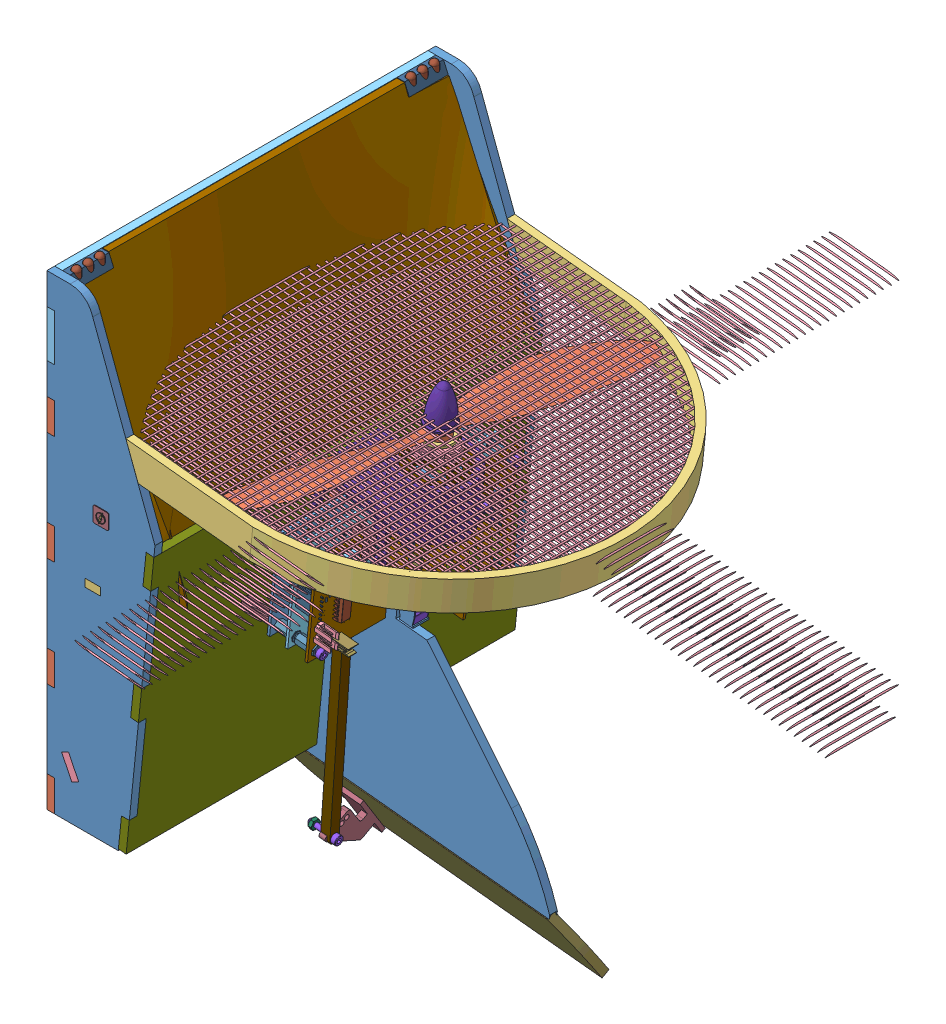
SolidWorks assembly AssTotaleSimu4, configuration Défaut. Lengths in mm. (continued)
Components (placement in the parent): (continued)
- AssStructSimu-1: AssStructSimu [Défaut] at (-125.7658 -1.8483 624.6548) x (1 0 0) z (0 0 -1) size (253.25 324.59 251.6) (continued)
  - AssCarte-1: AssCarte [Défaut] at (38.0121 147.1029 290.772) x (-0.101852 0.9948 0) z (0.9948 0.101852 0) size (66.52 130.57 98.72) (continued)
    - carte_onduleur_v3-1: carte_onduleur_v3 [Défaut] at (-131.8199 12.0892 20.7912) size (66.52 130.57 82.34) (continued)
      - U_DSPIC-1: U_DSPIC [Défaut] at (1.863 -2.61 0.803) size (7.92 35.56 7.75)
        - Open CASCADE STEP translator 6.8 1.17.1-1: Open CASCADE STEP translator 6.8 1.17.1 [Défaut] at origin size (7.92 35.56 7.75)
          - Body_1_4-1: Body_1_4 [Défaut] at (0 -0.2 4) x (1 0 0) z (0 -1 0) size (7.92 7.75 35.56)
      - C_DEC_DSPIC-1: C_DEC_DSPIC [Défaut] at (7.7 -8.8 -0.803) x (0 1 0) z (0 0 -1) size (2.34 1.04 0.5)
        - Open CASCADE STEP translator 6.8 1.6.1-1: Open CASCADE STEP translator 6.8 1.6.1 [Défaut] at origin size (2.34 1.04 0.5)
          - Body_1-1: Body_1 [Défaut] at origin size (2.29 1.04 0.43)
          - Pin_1-1: Pin_1 [Défaut] at (0.3048 0 0) x (-1 0 0) z (0 0 1) size (0.51 1.02 0.5)
          - Pin_2-1: Pin_2 [Défaut] at origin size (0.51 1.02 0.5)
      - IN-1: IN [Défaut] at (24.3 -5.3 0.803) x (0 1 0) z (0 0 1) size (10.21 15.56 26.9)
        - Open CASCADE STEP translator 6.8 1.19.1-1: Open CASCADE STEP translator 6.8 1.19.1 [Défaut] at origin size (10.21 15.56 26.9)
          - Body_1_3-1: Body_1_3 [Défaut] at (-13.5 1.8 3) x (0 1 0) z (1 0 0) size (15.56 26.9 10.21)
            - Imported-1: Imported [Défaut] at (2.0451 -4.5908 20.9802) size (8.6 15.9 10.16)
            - Imported-2: Imported [Défaut] at (-1.6683 9.1092 15.9802) x (0 0 1) z (-1 0 0) size (10.1 18.2 15.1)
              - Imported_2-1: Imported_2 [Défaut] at origin size (10.1 18.2 15.1)
              - Imported_3-1: Imported_3 [Défaut] at origin size (3.43 12.4 4.99)
              - Imported_4-1: Imported_4 [Défaut] at origin size (3.43 12.4 4.99)
              - Imported_5-1: Imported_5 [Défaut] at origin size (3.9 4.9 7)
              - Imported_6-1: Imported_6 [Défaut] at origin size (3.9 4.9 7)
              - Imported_7-1: Imported_7 [Défaut] at origin size (3.8 3.8 6.92)
              - Imported_8-1: Imported_8 [Défaut] at origin size (3.8 3.8 6.92)
              - Imported_9-1: Imported_9 [Défaut] at origin size (9 2.4 14.2)
      - CARTE_CMD-1: CARTE_CMD [Défaut] at (25 57.2 0.803) size (60.1 130 26.62)
        - Open CASCADE STEP translator 6.8 1.20.1-1: Open CASCADE STEP translator 6.8 1.20.1 [Défaut] at origin size (60.1 130 26.62)
          - Body_1_4-1: Body_1_4 [Défaut] at (-55 5 12) size (60.1 130 26.62)
            - 1_2-1: 1_2 [Défaut] at origin size (60.1 130 1.61)
            - 4-1: 4 [Défaut] at (23.6 -124.9 0.803) x (0 1 0) z (0 0 1) size (5 15.24 14.3)
              - =_[0_1_1_4]_2-1: =_[0_1_1_4]_2 [Défaut] at origin size (5 15.24 14.3)
                - 5-1: 5 [Défaut] at (0 -6.5 -13) x (0 1 0) z (0 0 -1) size (15.24 5 14.3)
            - 7-1: 7 [Défaut] at (23.6 -5 0.803) x (0 1 0) z (0 0 1) size (5 15.24 14.3)
              - =_[0_1_1_7]-1: =_[0_1_1_7] [Défaut] at origin size (5 15.24 14.3)
                - 5-1: 5 [Défaut] at (0 -6.5 -13) x (0 1 0) z (0 0 -1) size (15.24 5 14.3)
            - 10_2-1: 10_2 [Défaut] at (18.4 -115.6 0.803) size (25.4 7.92 7.75)
              - =_[0_1_1_9]-1: =_[0_1_1_9] [Défaut] at origin size (25.4 7.92 7.75)
                - 8-1: 8 [Défaut] at (11.2 4 0) x (0 1 0) z (1 0 0) size (7.92 7.75 25.4)
            - 13_2-1: 13_2 [Défaut] at (55.4 -114.7 0.803) x (-1 0 0) z (0 0 1) size (5 7.62 14.3)
              - =_[0_1_1_12]-1: =_[0_1_1_12] [Défaut] at origin size (5 7.62 14.3)
                - 11-1: 11 [Défaut] at (0 -2.5 11) x (0 -1 0) z (0 0 1) size (7.62 5 14.3)
            - 25-1: 25 [Défaut] at (56.9 -12.8 0.803) x (-1 0 0) z (0 0 1) size (16.02 47.26 11.05)
              - =_[0_1_1_15]_2-1: =_[0_1_1_15]_2 [Défaut] at origin size (16.02 47.26 11.05)
                - 23-1: 23 [Défaut] at (-36.5 21 4) x (0 -1 0) z (1 0 0) size (47.26 11.05 16.02)
                  - 14-1: 14 [Défaut] at (-7.4961 -1.5352 42.5833) size (42.58 6.55 16.01)
                  - 22-1: 22 [Défaut] at (19.3039 2.3748 37.905) x (-1 0 0) z (0 0 -1) size (10.36 6.14 15.24)
                    - 21-1: 21 [Défaut] at origin size (10.36 6.14 7.62)
                      - 19_2-1: 19_2 [Défaut] at origin size (10.36 6.14 2.54)
                        - 15-1: 15 [Défaut] at origin size (8.4 2.54 2.54)
                        - 16-1: 16 [Défaut] at (-0.0461 1.2682 1.27) x (0 0 -1) z (0.999998 -0.002105 0) size (1.95 5.07 7.58)
                      - 19_2-2: 19_2 [Défaut] at (0 0 -2.54) size (10.36 6.14 2.54)
                        - 15-1: 15 [Défaut] at origin size (8.4 2.54 2.54)
                        - 16-1: 16 [Défaut] at (-0.0461 1.2682 1.27) x (0 0 -1) z (0.999998 -0.002105 0) size (1.95 5.07 7.58)
                      - 19_2-3: 19_2 [Défaut] at (0 0 -5.08) size (10.36 6.14 2.54)
                        - 15-1: 15 [Défaut] at origin size (8.4 2.54 2.54)
                        - 16-1: 16 [Défaut] at (-0.0461 1.2682 1.27) x (0 0 -1) z (0.999998 -0.002105 0) size (1.95 5.07 7.58)
                    - 21-2: 21 [Défaut] at (0 0 -7.62) size (10.36 6.14 7.62)
                      - 19_2-1: 19_2 [Défaut] at origin size (10.36 6.14 2.54)
                        - 15-1: 15 [Défaut] at origin size (8.4 2.54 2.54)
                        - 16-1: 16 [Défaut] at (-0.0461 1.2682 1.27) x (0 0 -1) z (0.999998 -0.002105 0) size (1.95 5.07 7.58)
                      - 19_2-2: 19_2 [Défaut] at (0 0 -2.54) size (10.36 6.14 2.54)
                        - 15-1: 15 [Défaut] at origin size (8.4 2.54 2.54)
                        - 16-1: 16 [Défaut] at (-0.0461 1.2682 1.27) x (0 0 -1) z (0.999998 -0.002105 0) size (1.95 5.07 7.58)
                      - 19_2-3: 19_2 [Défaut] at (0 0 -5.08) size (10.36 6.14 2.54)
                        - 15-1: 15 [Défaut] at origin size (8.4 2.54 2.54)
                        - 16-1: 16 [Défaut] at (-0.0461 1.2682 1.27) x (0 0 -1) z (0.999998 -0.002105 0) size (1.95 5.07 7.58)
            - 31-1: 31 [Défaut] at (12.9 -104.5 0.803) size (6.76 3.64 4.37)
              - =_[0_1_1_24]-1: =_[0_1_1_24] [Défaut] at origin size (6.76 3.64 4.37)
                - 29-1: 29 [Défaut] at (-0.3 -2 0) size (6.76 3.64 4.37)
                  - =_[0_1_1_3]_3-1: =_[0_1_1_3]_3 [Défaut] at origin size (6 3.64 4.37)
                  - =_[0_1_1_4]_3-1: =_[0_1_1_4]_3 [Défaut] at origin size (0.38 1 0.67)
                  - =_[0_1_1_5]_3-1: =_[0_1_1_5]_3 [Défaut] at origin size (0.38 1 0.67)
            - 36-1: 36 [Défaut] at (28.6 -12.2 0.803) x (0 -1 0) z (0 0 1) size (2.34 1.04 0.5)
              - =_[0_1_1_30]-1: =_[0_1_1_30] [Défaut] at origin size (2.34 1.04 0.5)
                - 32_2-1: 32_2 [Défaut] at origin size (2.29 1.04 0.43)
                - 33_2-1: 33_2 [Défaut] at (0.3048 0 0) x (-1 0 0) z (0 0 1) size (0.51 1.02 0.5)
                - 34-1: 34 [Défaut] at origin size (0.51 1.02 0.5)
            - 38-1: 38 [Défaut] at (23.7 -12.2 0.803) x (0 -1 0) z (0 0 1) size (2.34 1.04 0.5)
              - =_[0_1_1_30]-1: =_[0_1_1_30] [Défaut] at origin size (2.34 1.04 0.5)
                - 32_2-1: 32_2 [Défaut] at origin size (2.29 1.04 0.43)
                - 33_2-1: 33_2 [Défaut] at (0.3048 0 0) x (-1 0 0) z (0 0 1) size (0.51 1.02 0.5)
                - 34-1: 34 [Défaut] at origin size (0.51 1.02 0.5)
            - 40_2-1: 40_2 [Défaut] at (26.2 -12.2 0.803) x (0 -1 0) z (0 0 1) size (2.34 1.04 0.5)
              - =_[0_1_1_30]-1: =_[0_1_1_30] [Défaut] at origin size (2.34 1.04 0.5)
                - 32_2-1: 32_2 [Défaut] at origin size (2.29 1.04 0.43)
                - 33_2-1: 33_2 [Défaut] at (0.3048 0 0) x (-1 0 0) z (0 0 1) size (0.51 1.02 0.5)
                - 34-1: 34 [Défaut] at origin size (0.51 1.02 0.5)
            - 42_2-1: 42_2 [Défaut] at (24.4 -119.2 0.803) size (2.34 1.04 0.5)
              - =_[0_1_1_30]-1: =_[0_1_1_30] [Défaut] at origin size (2.34 1.04 0.5)
                - 32_2-1: 32_2 [Défaut] at origin size (2.29 1.04 0.43)
                - 33_2-1: 33_2 [Défaut] at (0.3048 0 0) x (-1 0 0) z (0 0 1) size (0.51 1.02 0.5)
                - 34-1: 34 [Défaut] at origin size (0.51 1.02 0.5)
            - 45-1: 45 [Défaut] at (46.4 -125 0.803) size (5.08 5 14.3)
              - =_[0_1_1_38]-1: =_[0_1_1_38] [Défaut] at origin size (5.08 5 14.3)
                - 46-1: 46 [Défaut] at (1.2 0 11) size (5.08 5 14.3)
            - 48-1: 48 [Défaut] at (40.1 -125 0.803) size (5.08 5 14.3)
              - =_[0_1_1_41]-1: =_[0_1_1_41] [Défaut] at origin size (5.08 5 14.3)
                - 46-1: 46 [Défaut] at (1.2 0 11) size (5.08 5 14.3)
            - 51-1: 51 [Défaut] at (6.4 -119.9 0.803) x (0 1 0) z (0 0 1) size (15.24 2.54 7.37)
              - =_[0_1_1_43]-1: =_[0_1_1_43] [Défaut] at origin size (15.24 2.54 7.37)
                - 49_2-1: 49_2 [Défaut] at (6.5 0 0) x (1 0 0) z (0 -1 0) size (15.24 7.37 2.54)
            - 57_2-1: 57_2 [Défaut] at (50.8796 -121.1 -0.803) x (-1 0 0) z (0 0 -1) size (2.54 1.98 0.64)
              - =_[0_1_1_46]-1: =_[0_1_1_46] [Défaut] at origin size (2.54 1.98 0.64)
                - 52-1: 52 [Défaut] at origin size (2.54 1.14 0.58)
                - 53-1: 53 [Défaut] x (0 -1 0) z (0 0 1) size (0.43 0.51 0.38)
                - 54-1: 54 [Défaut] at (1.8796 1.8796 0) x (0 -1 0) z (0 0 1) size (0.43 0.51 0.38)
                - 55-1: 55 [Défaut] at (-0.9652 -2.8448 0) x (0 1 0) z (0 0 1) size (0.41 0.51 0.38)
            - 59_2-1: 59_2 [Défaut] at (43.6398 -120.995 -0.803) x (-1 0 0) z (0 0 -1) size (2.54 1.98 0.64)
              - =_[0_1_1_46]-1: =_[0_1_1_46] [Défaut] at origin size (2.54 1.98 0.64)
                - 52-1: 52 [Défaut] at origin size (2.54 1.14 0.58)
                - 53-1: 53 [Défaut] x (0 -1 0) z (0 0 1) size (0.43 0.51 0.38)
                - 54-1: 54 [Défaut] at (1.8796 1.8796 0) x (0 -1 0) z (0 0 1) size (0.43 0.51 0.38)
                - 55-1: 55 [Défaut] at (-0.9652 -2.8448 0) x (0 1 0) z (0 0 1) size (0.41 0.51 0.38)
            - 61_2-1: 61_2 [Défaut] at (47.6 -119.9 -0.803) x (-1 0 0) z (0 0 -1) size (2.34 1.04 0.5)
              - =_[0_1_1_30]-1: =_[0_1_1_30] [Défaut] at origin size (2.34 1.04 0.5)
                - 32_2-1: 32_2 [Défaut] at origin size (2.29 1.04 0.43)
                - 33_2-1: 33_2 [Défaut] at (0.3048 0 0) x (-1 0 0) z (0 0 1) size (0.51 1.02 0.5)
                - 34-1: 34 [Défaut] at origin size (0.51 1.02 0.5)
            - 63-1: 63 [Défaut] at (40.4 -119.9 -0.803) x (-1 0 0) z (0 0 -1) size (2.34 1.04 0.5)
              - =_[0_1_1_30]-1: =_[0_1_1_30] [Défaut] at origin size (2.34 1.04 0.5)
                - 32_2-1: 32_2 [Défaut] at origin size (2.29 1.04 0.43)
                - 33_2-1: 33_2 [Défaut] at (0.3048 0 0) x (-1 0 0) z (0 0 1) size (0.51 1.02 0.5)
                - 34-1: 34 [Défaut] at origin size (0.51 1.02 0.5)
            - 68-1: 68 [Défaut] at (47.7 -21.8 -0.803) x (0 1 0) z (0 0 -1) size (2.34 1.04 0.5)
              - =_[0_1_1_55]-1: =_[0_1_1_55] [Défaut] at origin size (2.34 1.04 0.5)
                - 64-1: 64 [Défaut] at origin size (2.29 1.04 0.43)
                - 65-1: 65 [Défaut] at (0.3048 0 0) x (-1 0 0) z (0 0 1) size (0.51 1.02 0.5)
                - 66-1: 66 [Défaut] at origin size (0.51 1.02 0.5)
            - 70-1: 70 [Défaut] at (47.6 -121.7 -0.803) x (-1 0 0) z (0 0 -1) size (2.34 1.04 0.5)
              - =_[0_1_1_30]-1: =_[0_1_1_30] [Défaut] at origin size (2.34 1.04 0.5)
                - 32_2-1: 32_2 [Défaut] at origin size (2.29 1.04 0.43)
                - 33_2-1: 33_2 [Défaut] at (0.3048 0 0) x (-1 0 0) z (0 0 1) size (0.51 1.02 0.5)
                - 34-1: 34 [Défaut] at origin size (0.51 1.02 0.5)
            - 72_2-1: 72_2 [Défaut] at (40.4 -121.5 -0.803) x (-1 0 0) z (0 0 -1) size (2.34 1.04 0.5)
              - =_[0_1_1_30]-1: =_[0_1_1_30] [Défaut] at origin size (2.34 1.04 0.5)
                - 32_2-1: 32_2 [Défaut] at origin size (2.29 1.04 0.43)
                - 33_2-1: 33_2 [Défaut] at (0.3048 0 0) x (-1 0 0) z (0 0 1) size (0.51 1.02 0.5)
                - 34-1: 34 [Défaut] at origin size (0.51 1.02 0.5)
            - 74_2-1: 74_2 [Défaut] at (47.7 -18.3 -0.803) x (0 1 0) z (0 0 -1) size (2.34 1.04 0.5)
              - =_[0_1_1_55]-1: =_[0_1_1_55] [Défaut] at origin size (2.34 1.04 0.5)
                - 64-1: 64 [Défaut] at origin size (2.29 1.04 0.43)
                - 65-1: 65 [Défaut] at (0.3048 0 0) x (-1 0 0) z (0 0 1) size (0.51 1.02 0.5)
                - 66-1: 66 [Défaut] at origin size (0.51 1.02 0.5)
            - 76_2-1: 76_2 [Défaut] at (45.5 -118.3 -0.803) x (1 0 0) z (0 0 -1) size (2.34 1.04 0.5)
              - =_[0_1_1_30]-1: =_[0_1_1_30] [Défaut] at origin size (2.34 1.04 0.5)
                - 32_2-1: 32_2 [Défaut] at origin size (2.29 1.04 0.43)
                - 33_2-1: 33_2 [Défaut] at (0.3048 0 0) x (-1 0 0) z (0 0 1) size (0.51 1.02 0.5)
                - 34-1: 34 [Défaut] at origin size (0.51 1.02 0.5)
            - 78_2-1: 78_2 [Défaut] at (38.2 -118.3 -0.803) x (1 0 0) z (0 0 -1) size (2.34 1.04 0.5)
              - =_[0_1_1_30]-1: =_[0_1_1_30] [Défaut] at origin size (2.34 1.04 0.5)
                - 32_2-1: 32_2 [Défaut] at origin size (2.29 1.04 0.43)
                - 33_2-1: 33_2 [Défaut] at (0.3048 0 0) x (-1 0 0) z (0 0 1) size (0.51 1.02 0.5)
                - 34-1: 34 [Défaut] at origin size (0.51 1.02 0.5)
            - 80_2-1: 80_2 [Défaut] at (28.6 -10.7 0.803) x (0 1 0) z (0 0 1) size (2.34 1.04 0.5)
              - =_[0_1_1_55]-1: =_[0_1_1_55] [Défaut] at origin size (2.34 1.04 0.5)
                - 64-1: 64 [Défaut] at origin size (2.29 1.04 0.43)
                - 65-1: 65 [Défaut] at (0.3048 0 0) x (-1 0 0) z (0 0 1) size (0.51 1.02 0.5)
                - 66-1: 66 [Défaut] at origin size (0.51 1.02 0.5)
            - 82_2-1: 82_2 [Défaut] at (23.7 -10.7 0.803) x (0 1 0) z (0 0 1) size (2.34 1.04 0.5)
              - =_[0_1_1_55]-1: =_[0_1_1_55] [Défaut] at origin size (2.34 1.04 0.5)
                - 64-1: 64 [Défaut] at origin size (2.29 1.04 0.43)
                - 65-1: 65 [Défaut] at (0.3048 0 0) x (-1 0 0) z (0 0 1) size (0.51 1.02 0.5)
                - 66-1: 66 [Défaut] at origin size (0.51 1.02 0.5)
            - 84-1: 84 [Défaut] at (26.2 -10.7 0.803) x (0 1 0) z (0 0 1) size (2.34 1.04 0.5)
              - =_[0_1_1_55]-1: =_[0_1_1_55] [Défaut] at origin size (2.34 1.04 0.5)
                - 64-1: 64 [Défaut] at origin size (2.29 1.04 0.43)
                - 65-1: 65 [Défaut] at (0.3048 0 0) x (-1 0 0) z (0 0 1) size (0.51 1.02 0.5)
                - 66-1: 66 [Défaut] at origin size (0.51 1.02 0.5)
            - 86-1: 86 [Défaut] at (23.0336 -119.2 0.803) x (-1 0 0) z (0 0 1) size (2.34 1.04 0.5)
              - =_[0_1_1_55]-1: =_[0_1_1_55] [Défaut] at origin size (2.34 1.04 0.5)
                - 64-1: 64 [Défaut] at origin size (2.29 1.04 0.43)
                - 65-1: 65 [Défaut] at (0.3048 0 0) x (-1 0 0) z (0 0 1) size (0.51 1.02 0.5)
                - 66-1: 66 [Défaut] at origin size (0.51 1.02 0.5)
            - 88-1: 88 [Défaut] at (14.1 -114.2 0.803) x (0 -1 0) z (0 0 1) size (2.34 1.04 0.5)
              - =_[0_1_1_55]-1: =_[0_1_1_55] [Défaut] at origin size (2.34 1.04 0.5)
                - 64-1: 64 [Défaut] at origin size (2.29 1.04 0.43)
                - 65-1: 65 [Défaut] at (0.3048 0 0) x (-1 0 0) z (0 0 1) size (0.51 1.02 0.5)
                - 66-1: 66 [Défaut] at origin size (0.51 1.02 0.5)
            - 90-1: 90 [Défaut] at (43.6 -107.8 -0.803) x (1 0 0) z (0 0 -1) size (2.34 1.04 0.5)
              - =_[0_1_1_55]-1: =_[0_1_1_55] [Défaut] at origin size (2.34 1.04 0.5)
                - 64-1: 64 [Défaut] at origin size (2.29 1.04 0.43)
                - 65-1: 65 [Défaut] at (0.3048 0 0) x (-1 0 0) z (0 0 1) size (0.51 1.02 0.5)
                - 66-1: 66 [Défaut] at origin size (0.51 1.02 0.5)
            - 92-1: 92 [Défaut] at (43.6 -106 -0.803) x (1 0 0) z (0 0 -1) size (2.34 1.04 0.5)
              - =_[0_1_1_55]-1: =_[0_1_1_55] [Défaut] at origin size (2.34 1.04 0.5)
                - 64-1: 64 [Défaut] at origin size (2.29 1.04 0.43)
                - 65-1: 65 [Défaut] at (0.3048 0 0) x (-1 0 0) z (0 0 1) size (0.51 1.02 0.5)
                - 66-1: 66 [Défaut] at origin size (0.51 1.02 0.5)
            - 175-1: 175 [Défaut] at (10 -21.7 0.803) x (0 -1 0) z (0 0 1) size (18.3 25.4 12.7)
              - =_[0_1_1_72]-1: =_[0_1_1_72] [Défaut] at origin size (18.3 25.4 12.7)
                - 173-1: 173 [Défaut] at (-1.4 -1 12) x (-1 0 0) z (0 1 0) size (18.3 12.7 25.4)
                  - board_1-1: board_1 [Défaut] at (-7.5 -1.57 12.5) size (15 1.57 25)
                  - hole_plating_20-1: hole_plating_20 [Défaut] at (-1.5 0 23.93) size (1.5 0.01 1.5)
                  - hole_plating_20-2: hole_plating_20 [Défaut] at (-1.5 0 21.39) size (1.5 0.01 1.5)
                  - hole_plating_20-3: hole_plating_20 [Défaut] at (-1.5 0 8.69) size (1.5 0.01 1.5)
                  - hole_plating_20-4: hole_plating_20 [Défaut] at (-1.5 -1.58 13.77) size (1.5 0.01 1.5)
                  - hole_plating_20-5: hole_plating_20 [Défaut] at (-1.5 0 16.31) size (1.5 0.01 1.5)
                  - hole_plating_20-6: hole_plating_20 [Défaut] at (-1.5 0 18.85) size (1.5 0.01 1.5)
                  - hole_plating_20-7: hole_plating_20 [Défaut] at (-1.5 0 13.77) size (1.5 0.01 1.5)
                  - hole_plating_20-8: hole_plating_20 [Défaut] at (-1.5 -1.58 11.23) size (1.5 0.01 1.5)
                  - hole_plating_20-9: hole_plating_20 [Défaut] at (-1.5 -1.58 18.85) size (1.5 0.01 1.5)
                  - hole_plating_20-10: hole_plating_20 [Défaut] at (-1.5 -1.58 6.15) size (1.5 0.01 1.5)
                  - hole_plating_20-11: hole_plating_20 [Défaut] at (-1.5 0 1.07) size (1.5 0.01 1.5)
                  - hole_plating_20-12: hole_plating_20 [Défaut] at (-1.5 -1.58 3.61) size (1.5 0.01 1.5)
                  - hole_plating_20-13: hole_plating_20 [Défaut] at (-1.5 -1.58 1.07) size (1.5 0.01 1.5)
                  - hole_plating_20-14: hole_plating_20 [Défaut] at (-1.5 -1.58 8.69) size (1.5 0.01 1.5)
                  - hole_plating_20-15: hole_plating_20 [Défaut] at (-1.5 -1.58 16.31) size (1.5 0.01 1.5)
                  - hole_plating_20-16: hole_plating_20 [Défaut] at (-1.5 0 11.23) size (1.5 0.01 1.5)
                  - hole_plating_20-17: hole_plating_20 [Défaut] at (-1.5 0 3.61) size (1.5 0.01 1.5)
                  - hole_plating_20-18: hole_plating_20 [Défaut] at (-1.5 -1.58 21.39) size (1.5 0.01 1.5)
                  - hole_plating_20-19: hole_plating_20 [Défaut] at (-1.5 0 6.15) size (1.5 0.01 1.5)
                  - hole_plating_20-20: hole_plating_20 [Défaut] at (-1.5 -1.58 23.93) size (1.5 0.01 1.5)
                  - Pin_Header_1x10_TH_Pitch_2.54mm_1-1: Pin_Header_1x10_TH_Pitch_2.54mm_1 [Défaut] at (-1.5 -1.5786 23.93) x (0 0 -1) z (0 -1 0) size (25.4 2.54 12.7)
                    - 124-1: 124 [Défaut] at origin size (25.4 2.54 2.8)
                      - =_[0_1_1_77]-1: =_[0_1_1_77] [Défaut] at origin size (2.54 2.54 2.8)
                      - =_[0_1_1_79]-1: =_[0_1_1_79] [Défaut] at origin size (2.54 2.54 2.8)
                      - =_[0_1_1_80]-1: =_[0_1_1_80] [Défaut] at origin size (2.54 2.54 2.8)
                      - =_[0_1_1_81]-1: =_[0_1_1_81] [Défaut] at origin size (2.54 2.54 2.8)
                      - =_[0_1_1_82]-1: =_[0_1_1_82] [Défaut] at origin size (2.54 2.54 2.8)
                      - =_[0_1_1_83]-1: =_[0_1_1_83] [Défaut] at origin size (2.54 2.54 2.8)
                      - =_[0_1_1_84]-1: =_[0_1_1_84] [Défaut] at origin size (2.54 2.54 2.8)
                      - =_[0_1_1_85]-1: =_[0_1_1_85] [Défaut] at origin size (2.54 2.54 2.8)
                      - =_[0_1_1_86]-1: =_[0_1_1_86] [Défaut] at origin size (2.54 2.54 2.8)
                      - =_[0_1_1_87]-1: =_[0_1_1_87] [Défaut] at origin size (2.54 2.54 2.8)
                    - 135-1: 135 [Défaut] at origin size (23.49 0.63 12.7)
                      - =_[0_1_1_88]-1: =_[0_1_1_88] [Défaut] at origin size (0.63 0.63 12.7)
                      - =_[0_1_1_90]-1: =_[0_1_1_90] [Défaut] at origin size (0.63 0.63 12.7)
                      - =_[0_1_1_91]-1: =_[0_1_1_91] [Défaut] at origin size (0.63 0.63 12.7)
                      - =_[0_1_1_92]-1: =_[0_1_1_92] [Défaut] at origin size (0.63 0.63 12.7)
                      - =_[0_1_1_93]-1: =_[0_1_1_93] [Défaut] at origin size (0.63 0.63 12.7)
                      - =_[0_1_1_94]-1: =_[0_1_1_94] [Défaut] at origin size (0.63 0.63 12.7)
                      - =_[0_1_1_95]-1: =_[0_1_1_95] [Défaut] at origin size (0.63 0.63 12.7)
                      - =_[0_1_1_96]-1: =_[0_1_1_96] [Défaut] at origin size (0.63 0.63 12.7)
                      - =_[0_1_1_97]-1: =_[0_1_1_97] [Défaut] at origin size (0.63 0.63 12.7)
                      - =_[0_1_1_98]-1: =_[0_1_1_98] [Défaut] at origin size (0.63 0.63 12.7)
                  - MPU-9250_1-1: MPU-9250_1 [Défaut] at (-8 0.05 12.5) x (-1 0 0) z (0 1 0) size (3 3 1.05)
                  - tantalum_10uF_1-1: tantalum_10uF_1 [Défaut] at (-13.167 0.1 10.9372) x (0 0 1) z (0 1 0) size (3.4 1.6 1.71)
                  - SOT23_5_1-1: SOT23_5_1 [Défaut] at (-7.475 -0.0136 21) x (0 0 1) z (0 1 0) size (3 3.2 0.92)
                  - RESC-0603_5-1: RESC-0603_5 [Défaut] at (-6.85 0 7.45) x (1 0 0) z (0 1 0) size (1.7 0.9 0.55)
                    - 143-1: 143 [Défaut] at origin size (1.7 0.9 0.55)
                      - =_[0_1_1_103]-1: =_[0_1_1_103] [Défaut] at origin size (0.4 0.9 0.53)
                      - =_[0_1_1_105]-1: =_[0_1_1_105] [Défaut] at origin size (0.4 0.9 0.53)
                      - =_[0_1_1_106]-1: =_[0_1_1_106] [Défaut] at origin size (1.64 0.9 0.52)
                    - 152-1: 152 [Défaut] at origin
                      - =_[0_1_1_107]-1: =_[0_1_1_107] [Défaut] at origin
                      - =_[0_1_1_109]-1: =_[0_1_1_109] [Défaut] at origin
                      - =_[0_1_1_110]-1: =_[0_1_1_110] [Défaut] at origin
                      - =_[0_1_1_111]-1: =_[0_1_1_111] [Défaut] at origin
                      - =_[0_1_1_112]-1: =_[0_1_1_112] [Défaut] at origin
                      - =_[0_1_1_113]-1: =_[0_1_1_113] [Défaut] at origin
                      - =_[0_1_1_114]-1: =_[0_1_1_114] [Défaut] at origin
                      - =_[0_1_1_115]-1: =_[0_1_1_115] [Défaut] at origin
                  - RESC-0603_5-2: RESC-0603_5 [Défaut] at (-9.85 0 16.05) x (1 0 0) z (0 1 0) size (1.7 0.9 0.55)
                    - 143-1: 143 [Défaut] at origin size (1.7 0.9 0.55)
                      - =_[0_1_1_103]-1: =_[0_1_1_103] [Défaut] at origin size (0.4 0.9 0.53)
                      - =_[0_1_1_105]-1: =_[0_1_1_105] [Défaut] at origin size (0.4 0.9 0.53)
                      - =_[0_1_1_106]-1: =_[0_1_1_106] [Défaut] at origin size (1.64 0.9 0.52)
                    - 152-1: 152 [Défaut] at origin
                      - =_[0_1_1_107]-1: =_[0_1_1_107] [Défaut] at origin
                      - =_[0_1_1_109]-1: =_[0_1_1_109] [Défaut] at origin
                      - =_[0_1_1_110]-1: =_[0_1_1_110] [Défaut] at origin
                      - =_[0_1_1_111]-1: =_[0_1_1_111] [Défaut] at origin
                      - =_[0_1_1_112]-1: =_[0_1_1_112] [Défaut] at origin
                      - =_[0_1_1_113]-1: =_[0_1_1_113] [Défaut] at origin
                      - =_[0_1_1_114]-1: =_[0_1_1_114] [Défaut] at origin
                      - =_[0_1_1_115]-1: =_[0_1_1_115] [Défaut] at origin
                  - RESC-0603_5-3: RESC-0603_5 [Défaut] at (-6.85 0 17.55) x (1 0 0) z (0 1 0) size (1.7 0.9 0.55)
                    - 143-1: 143 [Défaut] at origin size (1.7 0.9 0.55)
                      - =_[0_1_1_103]-1: =_[0_1_1_103] [Défaut] at origin size (0.4 0.9 0.53)
                      - =_[0_1_1_105]-1: =_[0_1_1_105] [Défaut] at origin size (0.4 0.9 0.53)
                      - =_[0_1_1_106]-1: =_[0_1_1_106] [Défaut] at origin size (1.64 0.9 0.52)
                    - 152-1: 152 [Défaut] at origin
                      - =_[0_1_1_107]-1: =_[0_1_1_107] [Défaut] at origin
                      - =_[0_1_1_109]-1: =_[0_1_1_109] [Défaut] at origin
                      - =_[0_1_1_110]-1: =_[0_1_1_110] [Défaut] at origin
                      - =_[0_1_1_111]-1: =_[0_1_1_111] [Défaut] at origin
                      - =_[0_1_1_112]-1: =_[0_1_1_112] [Défaut] at origin
                      - =_[0_1_1_113]-1: =_[0_1_1_113] [Défaut] at origin
                      - =_[0_1_1_114]-1: =_[0_1_1_114] [Défaut] at origin
                      - =_[0_1_1_115]-1: =_[0_1_1_115] [Défaut] at origin
                  - RESC-0603_5-4: RESC-0603_5 [Défaut] at (-6.85 0 16.05) x (1 0 0) z (0 1 0) size (1.7 0.9 0.55)
                    - 143-1: 143 [Défaut] at origin size (1.7 0.9 0.55)
                      - =_[0_1_1_103]-1: =_[0_1_1_103] [Défaut] at origin size (0.4 0.9 0.53)
                      - =_[0_1_1_105]-1: =_[0_1_1_105] [Défaut] at origin size (0.4 0.9 0.53)
                      - =_[0_1_1_106]-1: =_[0_1_1_106] [Défaut] at origin size (1.64 0.9 0.52)
                    - 152-1: 152 [Défaut] at origin
                      - =_[0_1_1_107]-1: =_[0_1_1_107] [Défaut] at origin
                      - =_[0_1_1_109]-1: =_[0_1_1_109] [Défaut] at origin
                      - =_[0_1_1_110]-1: =_[0_1_1_110] [Défaut] at origin
                      - =_[0_1_1_111]-1: =_[0_1_1_111] [Défaut] at origin
                      - =_[0_1_1_112]-1: =_[0_1_1_112] [Défaut] at origin
                      - =_[0_1_1_113]-1: =_[0_1_1_113] [Défaut] at origin
                      - =_[0_1_1_114]-1: =_[0_1_1_114] [Défaut] at origin
                      - =_[0_1_1_115]-1: =_[0_1_1_115] [Défaut] at origin
                  - RESC-0603_5-5: RESC-0603_5 [Défaut] at (-6.85 0 5.95) x (1 0 0) z (0 1 0) size (1.7 0.9 0.55)
                    - 143-1: 143 [Défaut] at origin size (1.7 0.9 0.55)
                      - =_[0_1_1_103]-1: =_[0_1_1_103] [Défaut] at origin size (0.4 0.9 0.53)
                      - =_[0_1_1_105]-1: =_[0_1_1_105] [Défaut] at origin size (0.4 0.9 0.53)
                      - =_[0_1_1_106]-1: =_[0_1_1_106] [Défaut] at origin size (1.64 0.9 0.52)
                    - 152-1: 152 [Défaut] at origin
                      - =_[0_1_1_107]-1: =_[0_1_1_107] [Défaut] at origin
                      - =_[0_1_1_109]-1: =_[0_1_1_109] [Défaut] at origin
                      - =_[0_1_1_110]-1: =_[0_1_1_110] [Défaut] at origin
                      - =_[0_1_1_111]-1: =_[0_1_1_111] [Défaut] at origin
                      - =_[0_1_1_112]-1: =_[0_1_1_112] [Défaut] at origin
                      - =_[0_1_1_113]-1: =_[0_1_1_113] [Défaut] at origin
                      - =_[0_1_1_114]-1: =_[0_1_1_114] [Défaut] at origin
                      - =_[0_1_1_115]-1: =_[0_1_1_115] [Défaut] at origin
                  - CAPC-0603-T0.9-BN_5-1: CAPC-0603-T0.9-BN_5 [Défaut] at (-9.85 0 8.95) x (1 0 0) z (0 1 0) size (1.7 0.9 0.9)
                    - =_[0_1_1_117]-1: =_[0_1_1_117] [Défaut] at origin size (1.7 0.9 0.9)
                    - 167-1: 167 [Défaut] at origin
                      - =_[0_1_1_118]-1: =_[0_1_1_118] [Défaut] at origin
                      - =_[0_1_1_120]-1: =_[0_1_1_120] [Défaut] at origin
                      - =_[0_1_1_121]-1: =_[0_1_1_121] [Défaut] at origin
                      - =_[0_1_1_122]-1: =_[0_1_1_122] [Défaut] at origin
                      - =_[0_1_1_123]-1: =_[0_1_1_123] [Défaut] at origin
                      - =_[0_1_1_124]-1: =_[0_1_1_124] [Défaut] at origin
                      - =_[0_1_1_125]-1: =_[0_1_1_125] [Défaut] at origin
                      - =_[0_1_1_126]-1: =_[0_1_1_126] [Défaut] at origin
                  - CAPC-0603-T0.9-BN_5-2: CAPC-0603-T0.9-BN_5 [Défaut] at (-6.85 0 8.95) x (1 0 0) z (0 1 0) size (1.7 0.9 0.9)
                    - =_[0_1_1_117]-1: =_[0_1_1_117] [Défaut] at origin size (1.7 0.9 0.9)
                    - 167-1: 167 [Défaut] at origin
                      - =_[0_1_1_118]-1: =_[0_1_1_118] [Défaut] at origin
                      - =_[0_1_1_120]-1: =_[0_1_1_120] [Défaut] at origin
                      - =_[0_1_1_121]-1: =_[0_1_1_121] [Défaut] at origin
                      - =_[0_1_1_122]-1: =_[0_1_1_122] [Défaut] at origin
                      - =_[0_1_1_123]-1: =_[0_1_1_123] [Défaut] at origin
                      - =_[0_1_1_124]-1: =_[0_1_1_124] [Défaut] at origin
                      - =_[0_1_1_125]-1: =_[0_1_1_125] [Défaut] at origin
                      - =_[0_1_1_126]-1: =_[0_1_1_126] [Défaut] at origin
                  - CAPC-0603-T0.9-BN_5-3: CAPC-0603-T0.9-BN_5 [Défaut] at (-6.85 0 19.05) x (1 0 0) z (0 1 0) size (1.7 0.9 0.9)
                    - =_[0_1_1_117]-1: =_[0_1_1_117] [Défaut] at origin size (1.7 0.9 0.9)
                    - 167-1: 167 [Défaut] at origin
                      - =_[0_1_1_118]-1: =_[0_1_1_118] [Défaut] at origin
                      - =_[0_1_1_120]-1: =_[0_1_1_120] [Défaut] at origin
                      - =_[0_1_1_121]-1: =_[0_1_1_121] [Défaut] at origin
                      - =_[0_1_1_122]-1: =_[0_1_1_122] [Défaut] at origin
                      - =_[0_1_1_123]-1: =_[0_1_1_123] [Défaut] at origin
                      - =_[0_1_1_124]-1: =_[0_1_1_124] [Défaut] at origin
                      - =_[0_1_1_125]-1: =_[0_1_1_125] [Défaut] at origin
                      - =_[0_1_1_126]-1: =_[0_1_1_126] [Défaut] at origin
                  - CAPC-0603-T0.9-BN_5-4: CAPC-0603-T0.9-BN_5 [Défaut] at (-9.85 0 7.45) x (1 0 0) z (0 1 0) size (1.7 0.9 0.9)
                    - =_[0_1_1_117]-1: =_[0_1_1_117] [Défaut] at origin size (1.7 0.9 0.9)
                    - 167-1: 167 [Défaut] at origin
                      - =_[0_1_1_118]-1: =_[0_1_1_118] [Défaut] at origin
                      - =_[0_1_1_120]-1: =_[0_1_1_120] [Défaut] at origin
                      - =_[0_1_1_121]-1: =_[0_1_1_121] [Défaut] at origin
                      - =_[0_1_1_122]-1: =_[0_1_1_122] [Défaut] at origin
                      - =_[0_1_1_123]-1: =_[0_1_1_123] [Défaut] at origin
                      - =_[0_1_1_124]-1: =_[0_1_1_124] [Défaut] at origin
                      - =_[0_1_1_125]-1: =_[0_1_1_125] [Défaut] at origin
                      - =_[0_1_1_126]-1: =_[0_1_1_126] [Défaut] at origin
                  - CAPC-0603-T0.9-BN_5-5: CAPC-0603-T0.9-BN_5 [Défaut] at (-9.85 0 17.55) x (1 0 0) z (0 1 0) size (1.7 0.9 0.9)
                    - =_[0_1_1_117]-1: =_[0_1_1_117] [Défaut] at origin size (1.7 0.9 0.9)
                    - 167-1: 167 [Défaut] at origin
                      - =_[0_1_1_118]-1: =_[0_1_1_118] [Défaut] at origin
                      - =_[0_1_1_120]-1: =_[0_1_1_120] [Défaut] at origin
                      - =_[0_1_1_121]-1: =_[0_1_1_121] [Défaut] at origin
                      - =_[0_1_1_122]-1: =_[0_1_1_122] [Défaut] at origin
                      - =_[0_1_1_123]-1: =_[0_1_1_123] [Défaut] at origin
                      - =_[0_1_1_124]-1: =_[0_1_1_124] [Défaut] at origin
                      - =_[0_1_1_125]-1: =_[0_1_1_125] [Défaut] at origin
                      - =_[0_1_1_126]-1: =_[0_1_1_126] [Défaut] at origin
            - 177-1: 177 [Défaut] at (52.1 -16.5 -0.803) x (1 0 0) z (0 0 -1) size (2.34 1.04 0.5)
              - =_[0_1_1_30]-1: =_[0_1_1_30] [Défaut] at origin size (2.34 1.04 0.5)
                - 32_2-1: 32_2 [Défaut] at origin size (2.29 1.04 0.43)
                - 33_2-1: 33_2 [Défaut] at (0.3048 0 0) x (-1 0 0) z (0 0 1) size (0.51 1.02 0.5)
                - 34-1: 34 [Défaut] at origin size (0.51 1.02 0.5)
            - 179-1: 179 [Défaut] at (22.5336 -121.5 -0.803) x (-1 0 0) z (0 0 -1) size (2.34 1.04 0.5)
              - =_[0_1_1_30]-1: =_[0_1_1_30] [Défaut] at origin size (2.34 1.04 0.5)
                - 32_2-1: 32_2 [Défaut] at origin size (2.29 1.04 0.43)
                - 33_2-1: 33_2 [Défaut] at (0.3048 0 0) x (-1 0 0) z (0 0 1) size (0.51 1.02 0.5)
                - 34-1: 34 [Défaut] at origin size (0.51 1.02 0.5)
            - 181-1: 181 [Défaut] at (48.6 -127 -0.803) x (-1 0 0) z (0 0 -1) size (2.34 1.04 0.5)
              - =_[0_1_1_30]-1: =_[0_1_1_30] [Défaut] at origin size (2.34 1.04 0.5)
                - 32_2-1: 32_2 [Défaut] at origin size (2.29 1.04 0.43)
                - 33_2-1: 33_2 [Défaut] at (0.3048 0 0) x (-1 0 0) z (0 0 1) size (0.51 1.02 0.5)
                - 34-1: 34 [Défaut] at origin size (0.51 1.02 0.5)
            - 183-1: 183 [Défaut] at (26.0189 -121.5 0.803) size (2.34 1.04 0.5)
              - =_[0_1_1_30]-1: =_[0_1_1_30] [Défaut] at origin size (2.34 1.04 0.5)
                - 32_2-1: 32_2 [Défaut] at origin size (2.29 1.04 0.43)
                - 33_2-1: 33_2 [Défaut] at (0.3048 0 0) x (-1 0 0) z (0 0 1) size (0.51 1.02 0.5)
                - 34-1: 34 [Défaut] at origin size (0.51 1.02 0.5)
            - 185-1: 185 [Défaut] at (30.3664 -19 -0.803) x (1 0 0) z (0 0 -1) size (2.34 1.04 0.5)
              - =_[0_1_1_30]-1: =_[0_1_1_30] [Défaut] at origin size (2.34 1.04 0.5)
                - 32_2-1: 32_2 [Défaut] at origin size (2.29 1.04 0.43)
                - 33_2-1: 33_2 [Défaut] at (0.3048 0 0) x (-1 0 0) z (0 0 1) size (0.51 1.02 0.5)
                - 34-1: 34 [Défaut] at origin size (0.51 1.02 0.5)
            - 187-1: 187 [Défaut] at (51.7 -114.3 -0.803) x (0 1 0) z (0 0 -1) size (2.34 1.04 0.5)
              - =_[0_1_1_30]-1: =_[0_1_1_30] [Défaut] at origin size (2.34 1.04 0.5)
                - 32_2-1: 32_2 [Défaut] at origin size (2.29 1.04 0.43)
                - 33_2-1: 33_2 [Défaut] at (0.3048 0 0) x (-1 0 0) z (0 0 1) size (0.51 1.02 0.5)
                - 34-1: 34 [Défaut] at origin size (0.51 1.02 0.5)
            - 189-1: 189 [Défaut] at (50 -114.3 -0.803) x (0 1 0) z (0 0 -1) size (2.34 1.04 0.5)
              - =_[0_1_1_30]-1: =_[0_1_1_30] [Défaut] at origin size (2.34 1.04 0.5)
                - 32_2-1: 32_2 [Défaut] at origin size (2.29 1.04 0.43)
                - 33_2-1: 33_2 [Défaut] at (0.3048 0 0) x (-1 0 0) z (0 0 1) size (0.51 1.02 0.5)
                - 34-1: 34 [Défaut] at origin size (0.51 1.02 0.5)
      - C2_1-1: C2_1 [Défaut] at (-20.6984 1.8 -0.803) x (1 0 0) z (0 0 -1) size (2.34 1.04 0.5)
        - Open CASCADE STEP translator 6.8 1.6.1-1: Open CASCADE STEP translator 6.8 1.6.1 [Défaut] at origin size (2.34 1.04 0.5)
          - Body_1-1: Body_1 [Défaut] at origin size (2.29 1.04 0.43)
          - Pin_1-1: Pin_1 [Défaut] at (0.3048 0 0) x (-1 0 0) z (0 0 1) size (0.51 1.02 0.5)
          - Pin_2-1: Pin_2 [Défaut] at origin size (0.51 1.02 0.5)
      - C2_2-1: C2_2 [Défaut] at (-24.2 1.8 -0.803) x (1 0 0) z (0 0 -1) size (2.34 1.04 0.5)
        - Open CASCADE STEP translator 6.8 1.6.1-1: Open CASCADE STEP translator 6.8 1.6.1 [Défaut] at origin size (2.34 1.04 0.5)
          - Body_1-1: Body_1 [Défaut] at origin size (2.29 1.04 0.43)
          - Pin_1-1: Pin_1 [Défaut] at (0.3048 0 0) x (-1 0 0) z (0 0 1) size (0.51 1.02 0.5)
          - Pin_2-1: Pin_2 [Défaut] at origin size (0.51 1.02 0.5)
      - C3_1-1: C3_1 [Défaut] at (-20.9176 -12.8 -0.803) x (1 0 0) z (0 0 -1) size (2.34 1.04 0.5)
        - Open CASCADE STEP translator 6.8 1.6.1-1: Open CASCADE STEP translator 6.8 1.6.1 [Défaut] at origin size (2.34 1.04 0.5)
          - Body_1-1: Body_1 [Défaut] at origin size (2.29 1.04 0.43)
          - Pin_1-1: Pin_1 [Défaut] at (0.3048 0 0) x (-1 0 0) z (0 0 1) size (0.51 1.02 0.5)
          - Pin_2-1: Pin_2 [Défaut] at origin size (0.51 1.02 0.5)
      - C3_2-1: C3_2 [Défaut] at (-24.4 -12.8 -0.803) x (1 0 0) z (0 0 -1) size (2.34 1.04 0.5)
        - Open CASCADE STEP translator 6.8 1.6.1-1: Open CASCADE STEP translator 6.8 1.6.1 [Défaut] at origin size (2.34 1.04 0.5)
          - Body_1-1: Body_1 [Défaut] at origin size (2.29 1.04 0.43)
          - Pin_1-1: Pin_1 [Défaut] at (0.3048 0 0) x (-1 0 0) z (0 0 1) size (0.51 1.02 0.5)
          - Pin_2-1: Pin_2 [Défaut] at origin size (0.51 1.02 0.5)
      - D_CUR-1: D_CUR [Défaut] at (-12.4432 3.85 -0.803) x (0 -1 0) z (0 0 -1) size (2.7 5.2 1.11)
        - Open CASCADE STEP translator 6.8 1.25.1-1: Open CASCADE STEP translator 6.8 1.25.1 [Défaut] at origin size (2.7 5.2 1.11)
          - Body_1_5-1: Body_1_5 [Défaut] at (1.2 -4 0) x (0 1 0) z (0 0 1) size (5.2 2.7 1.11)
            - =_[0_1_1_3]_4-1: =_[0_1_1_3]_4 [Défaut] at origin size (0.39 0.64 0.01)
            - =_[0_1_1_4]_4-1: =_[0_1_1_4]_4 [Défaut] at origin size (0.6 1.9 0.2)
            - =_[0_1_1_5]_4-1: =_[0_1_1_5]_4 [Défaut] at origin size (0.21 0.08 0.01)
            - =_[0_1_1_6]_2-1: =_[0_1_1_6]_2 [Défaut] at origin size (0.6 1.9 0.2)
            - =_[0_1_1_7]_2-1: =_[0_1_1_7]_2 [Défaut] at origin size (0.46 0.68 0.01)
            - =_[0_1_1_8]_2-1: =_[0_1_1_8]_2 [Défaut] at origin size (0.38 0.66 0.01)
            - =_[0_1_1_9]-1: =_[0_1_1_9] [Défaut] at origin size (0.2 0.62 0.01)
            - =_[0_1_1_10]-1: =_[0_1_1_10] [Défaut] at origin size (4 2.7 1.1)
            - =_[0_1_1_11]-1: =_[0_1_1_11] [Défaut] at origin size (0.46 0.63 0.01)
            - =_[0_1_1_12]-1: =_[0_1_1_12] [Défaut] at origin size (0.56 0.68 0.01)
      - RC1_1-1: RC1_1 [Défaut] at (-20.7176 8.1 -0.803) x (1 0 0) z (0 0 -1) size (2.34 1.04 0.5)
        - Open CASCADE STEP translator 6.8 1.12.1-1: Open CASCADE STEP translator 6.8 1.12.1 [Défaut] at origin size (2.34 1.04 0.5)
          - Body_1_3-1: Body_1_3 [Défaut] at origin size (2.29 1.04 0.43)
          - Pin_1_2-1: Pin_1_2 [Défaut] at (0.3048 0 0) x (-1 0 0) z (0 0 1) size (0.51 1.02 0.5)
          - Pin_2_2-1: Pin_2_2 [Défaut] at origin size (0.51 1.02 0.5)
      - RC1_2-1: RC1_2 [Défaut] at (-22 8.1 -0.803) x (-1 0 0) z (0 0 -1) size (2.34 1.04 0.5)
        - Open CASCADE STEP translator 6.8 1.12.1-1: Open CASCADE STEP translator 6.8 1.12.1 [Défaut] at origin size (2.34 1.04 0.5)
          - Body_1_3-1: Body_1_3 [Défaut] at origin size (2.29 1.04 0.43)
          - Pin_1_2-1: Pin_1_2 [Défaut] at (0.3048 0 0) x (-1 0 0) z (0 0 1) size (0.51 1.02 0.5)
          - Pin_2_2-1: Pin_2_2 [Défaut] at origin size (0.51 1.02 0.5)
      - RC2_1-1: RC2_1 [Défaut] at (-20.716 0.243 -0.803) x (1 0 0) z (0 0 -1) size (2.34 1.04 0.5)
        - Open CASCADE STEP translator 6.8 1.12.1-1: Open CASCADE STEP translator 6.8 1.12.1 [Défaut] at origin size (2.34 1.04 0.5)
          - Body_1_3-1: Body_1_3 [Défaut] at origin size (2.29 1.04 0.43)
          - Pin_1_2-1: Pin_1_2 [Défaut] at (0.3048 0 0) x (-1 0 0) z (0 0 1) size (0.51 1.02 0.5)
          - Pin_2_2-1: Pin_2_2 [Défaut] at origin size (0.51 1.02 0.5)
      - RC2_2-1: RC2_2 [Défaut] at (-22 0.18 -0.803) x (-1 0 0) z (0 0 -1) size (2.34 1.04 0.5)
        - Open CASCADE STEP translator 6.8 1.12.1-1: Open CASCADE STEP translator 6.8 1.12.1 [Défaut] at origin size (2.34 1.04 0.5)
          - Body_1_3-1: Body_1_3 [Défaut] at origin size (2.29 1.04 0.43)
          - Pin_1_2-1: Pin_1_2 [Défaut] at (0.3048 0 0) x (-1 0 0) z (0 0 1) size (0.51 1.02 0.5)
